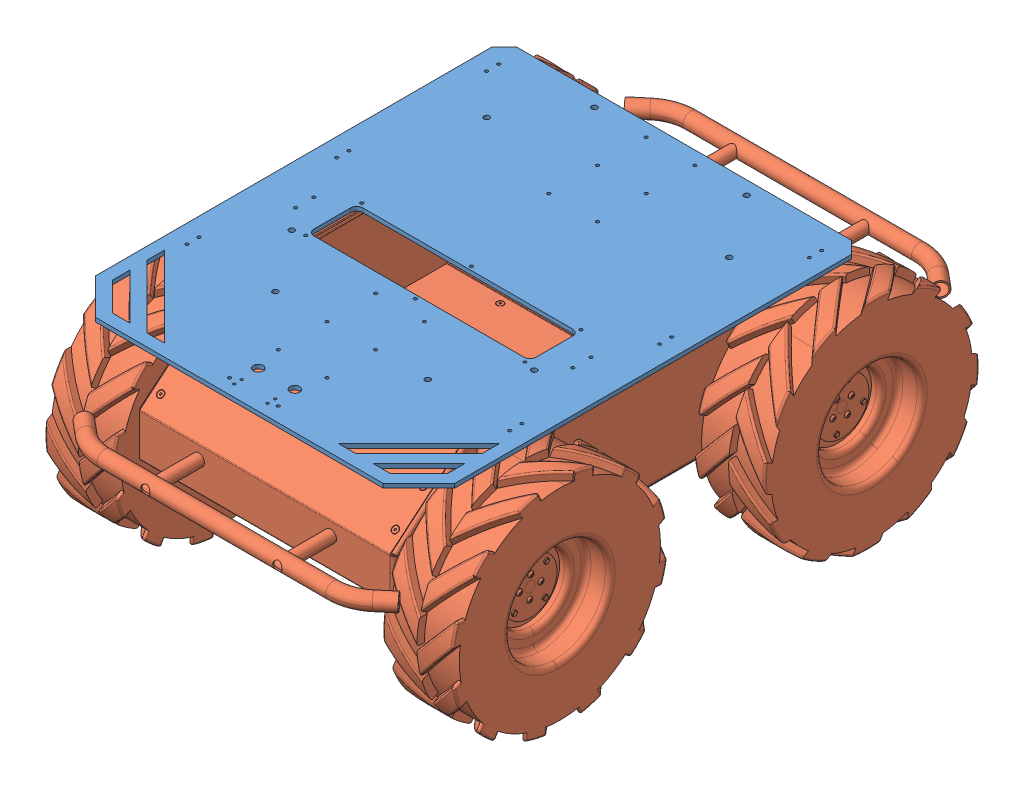
SolidWorks assembly plate on husky, configuration Default. Lengths in mm.
Overall size (675.09 407.82 987.47).
2 component instances, 2 part files, 6 mates.
Components (placement in the parent):
- baseplate2-1: baseplate2 [Default] at (0 244.325 82.6976) x (-1 0 0) z (0 0 -1) size (590 6.7 730)
- husky-1: husky [Default] at origin size (675.09 404.16 987.47)
Mates (geometry in assembly coordinates):
- Coincident1: coincident aligned: plane of husky-1 through (0 0 0) normal (1 0 0)
- Coincident2: coincident aligned: plane of husky-1 through (0 0 0) normal (0 1 0)
- Coincident3: coincident aligned: plane of husky-1 through (0 0 0) normal (0 0 1)
- Coincident5: coincident aligned: plane of baseplate2-1 through (0 244.325 107.6976) normal (0 -1 0)
- Distance2: distance = 85 mm: plane of assembly; plane of assembly; plane of baseplate2-1 through (295 251.025 82.6976) normal (1 0 0)
- Distance3: distance = 175 mm: plane of assembly; plane of assembly; plane of baseplate2-1 through (0 251.025 447.6976) normal (0 0 1)
